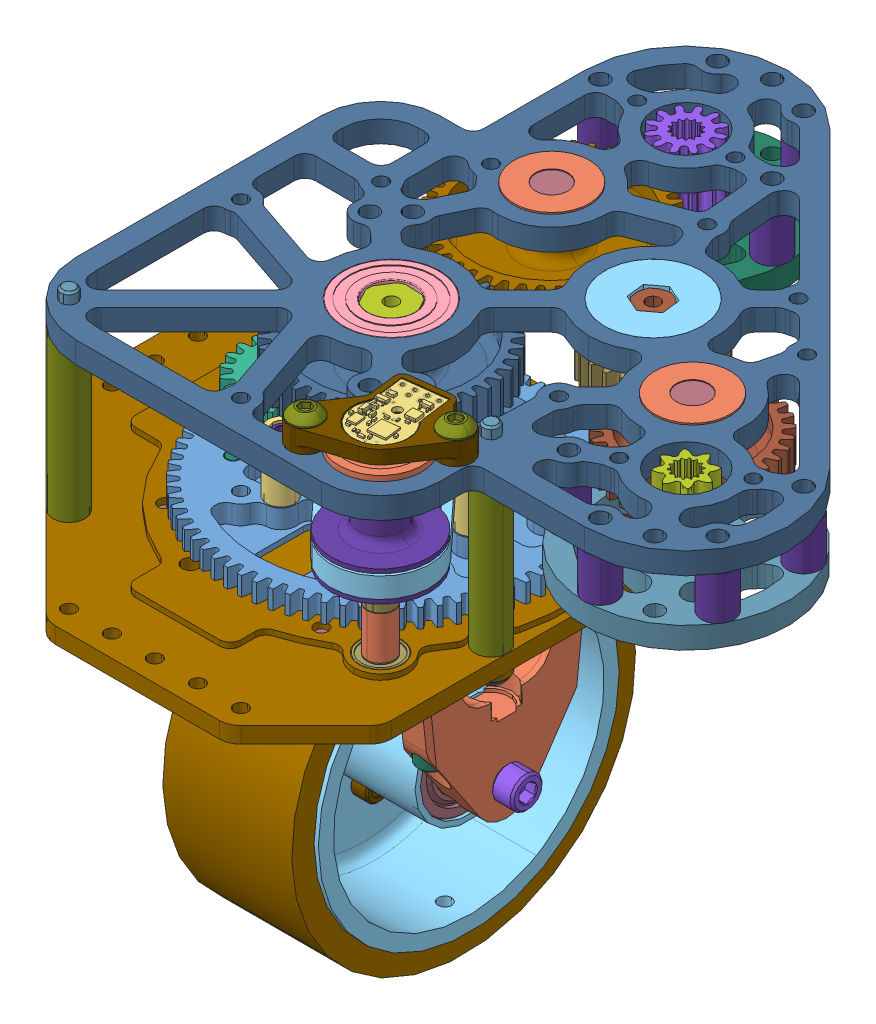
SolidWorks assembly WCP-0361 - Swerve X (Tube Mount, Flipped Gears Below) (WCP-0363).step-1, configuration Default. Lengths in mm.
Overall size (208.72 184.42 201.03).
94 component instances, 59 part files, 0 mates.
Components (placement in the parent):
- WCP-0364 Rev1 - WCP X Wheel Module.step-1-1: WCP-0364 Rev1 - WCP X Wheel Module.step-1 [Default] at (0 -0.825 0) size (95.62 174.54 137.74)
  - WCP-0364-001 Rev1.step-1-1: WCP-0364-001 Rev1.step-1 [Default] at (0 6.35 0) size (93.93 9.53 93.93)
  - WCP-0366 Rev1_Default_As Machined_.step-1-1: WCP-0366 Rev1_Default_As Machined_.step-1 [Default] at (29.2862 -49.2125 0) x (0 0 -1) z (1 0 0) size (51.81 60.46 9.5)
  - WCP-0366 Rev1_Default_As Machined_.step-1-2: WCP-0366 Rev1_Default_As Machined_.step-1 [Default] at (-29.2862 -49.2125 0) x (0 0 1) z (-1 0 0) size (51.81 60.46 9.5)
  - WCP-0364-006 Rev1.step-1-1: WCP-0364-006 Rev1.step-1 [Default] at (0 -49.2125 0) x (1 0 0) z (0 -0.837962 0.545729) size (56.46 12.67 12.67)
  - WCP-0364-005 Rev2.step-1-1: WCP-0364-005 Rev2.step-1 [Default] at (-29.2862 -1.2827 0) x (0 -1 0) z (0 0 1) size (54.08 11 11)
  - WCP-0365 Rev2.step-1-1: WCP-0365 Rev2.step-1 [Default] at (2.3061 -49.2125 0) x (0 -0.866025 -0.5) z (1 0 0) size (88.9 88.9 41.15)
  - WCP-0233 Rev1.step-1-1: WCP-0233 Rev1.step-1 [Default] at (-18.0375 -49.2125 0) x (0 0 -1) z (0 1 0) size (68.52 16.32 68.56)
  - WCP-0364-002 Rev1.step-1-1: WCP-0364-002 Rev1.step-1 [Default] at (0 34.5757 0) x (0 -1 0) z (0.999257 0 0.03854) size (51.69 15 15)
  - WCP-0276 Rev1.step-1-1: WCP-0276 Rev1.step-1 [Default] at (-29.2862 -15.4625 0) x (0 0 1) z (1 0 0) size (25.2 12.86 25.34)
  - WCP-0364-008 Rev1.step-1-1: WCP-0364-008 Rev1.step-1 [Default] at (2.3061 -49.2125 0) x (1 0 0) z (0 -0.879106 0.476626) size (38.1 101.6 101.6)
  - WCP-0357 Rev1.step-1-1: WCP-0357 Rev1.step-1 [Default] at origin size (88.91 6.35 88.9)
  - 217-5829_0375_flanged_thunderhex_bearing.step-1-1: 217-5829_0375_flanged_thunderhex_bearing.step-1 [Default] at (-29.2862 12.7 0) x (0 -1 0) z (0.06043 0 0.998172) size (7.11 24.61 24.61)
  - 217-3489_0_250_radial_bearing.step-1-1: 217-3489_0_250_radial_bearing.step-1 [Default] at (-29.2862 -29.3687 0) x (0 -1 0) z (0.460874 0 0.887465) size (4.76 12.7 12.7)
  - 217-3109_0_500_radial_bearing.step-1-1: 217-3109_0_500_radial_bearing.step-1 [Default] at (-17.8424 -49.2125 0) x (1 0 0) z (0 0.040496 0.99918) size (7.94 28.57 28.57)
  - 217-3109_0_500_radial_bearing.step-1-2: 217-3109_0_500_radial_bearing.step-1 [Default] at (18.0604 -49.2125 0) x (1 0 0) z (0 -0.205758 0.978603) size (7.94 28.57 28.57)
  - 217-2731_0_500_flanged_bearing.step-1-1: 217-2731_0_500_flanged_bearing.step-1 [Default] at (0 4.7625 0) x (0.999376 0 -0.035335) z (0.035335 0 0.999376) size (31.12 7.94 31.12)
  - NFS-0018_SHCS_#10-32_1_750L_Default_As Machined_.step-1-1: NFS-0018_SHCS_#10-32_1_750L_Default_As Machined_.step-1 [Default] at (-29.2862 11.1125 17.4625) x (0.988526 0 -0.151053) z (0 1 0) size (7.92 7.92 49.28)
  - NFS-0018_SHCS_#10-32_1_750L_Default_As Machined_.step-1-2: NFS-0018_SHCS_#10-32_1_750L_Default_As Machined_.step-1 [Default] at (-29.2862 11.1125 -17.4625) x (0.988526 0 -0.151053) z (0 1 0) size (7.92 7.92 49.28)
  - NFS-0018_SHCS_#10-32_1_750L_Default_As Machined_.step-1-3: NFS-0018_SHCS_#10-32_1_750L_Default_As Machined_.step-1 [Default] at (29.2862 11.1125 17.4625) x (0.988526 0 -0.151053) z (0 1 0) size (7.92 7.92 49.28)
  - NFS-0018_SHCS_#10-32_1_750L_Default_As Machined_.step-1-4: NFS-0018_SHCS_#10-32_1_750L_Default_As Machined_.step-1 [Default] at (29.2862 11.1125 -17.4625) x (0.988526 0 -0.151053) z (0 1 0) size (7.92 7.92 49.28)
  - 8-32 BHCS_0.500.step-1-1: 8-32 BHCS_0.500.step-1 [Default] at (-29.2862 23.8633 0) x (0.940105 0 -0.340884) z (0.340884 0 0.940105) size (7.92 14.92 7.92)
  - NFS-0059_SHCS_#4-40_0_875L_91251A113.step-1-1: NFS-0059_SHCS_#4-40_0_875L_91251A113.step-1 [Default] at (23.876 3.5687 0) x (0.431119 0 0.902295) z (0 -1 0) size (4.65 4.65 25.08)
  - NFS-0059_SHCS_#4-40_0_875L_91251A113.step-1-2: NFS-0059_SHCS_#4-40_0_875L_91251A113.step-1 [Default] at (23.876 3.0654 0) x (0.520663 0 0.853762) z (0 -1 0) size (4.65 4.65 25.08)
  - NFS-0059_SHCS_#4-40_0_875L_91251A113.step-1-3: NFS-0059_SHCS_#4-40_0_875L_91251A113.step-1 [Default] at (-11.938 3.5687 -20.6772) x (0.431119 0 0.902295) z (0 -1 0) size (4.65 4.65 25.08)
  - NFS-0059_SHCS_#4-40_0_875L_91251A113.step-1-4: NFS-0059_SHCS_#4-40_0_875L_91251A113.step-1 [Default] at (-11.938 3.0654 -20.6772) x (0.520663 0 0.853762) z (0 -1 0) size (4.65 4.65 25.08)
  - NFS-0059_SHCS_#4-40_0_875L_91251A113.step-1-5: NFS-0059_SHCS_#4-40_0_875L_91251A113.step-1 [Default] at (-11.938 3.0654 20.6772) x (0.520663 0 0.853762) z (0 -1 0) size (4.65 4.65 25.08)
  - 10-32 SHCS - No Thread_WCP-0265 - 0.375.step-1-1: 10-32 SHCS - No Thread_WCP-0265 - 0.375.step-1 [Default] at (-8.2862 -59.5312 17.8726) x (0 -0.796051 -0.60523) z (0 -0.60523 0.796051) size (7.67 14.35 7.67)
  - 10-32 SHCS - No Thread_WCP-0265 - 0.375.step-1-2: 10-32 SHCS - No Thread_WCP-0265 - 0.375.step-1 [Default] at (-8.2862 -38.8937 -17.8726) x (0 -0.796051 -0.60523) z (0 -0.60523 0.796051) size (7.67 14.35 7.67)
  - 10-32 SHCS - No Thread_WCP-0265 - 0.375.step-1-3: 10-32 SHCS - No Thread_WCP-0265 - 0.375.step-1 [Default] at (-8.2862 -38.8937 17.8726) x (0 -0.796051 -0.60523) z (0 -0.60523 0.796051) size (7.67 14.35 7.67)
  - 10-32 SHCS - No Thread_WCP-0265 - 0.375.step-1-4: 10-32 SHCS - No Thread_WCP-0265 - 0.375.step-1 [Default] at (-8.2862 -59.5312 -17.8726) x (0 -0.796051 -0.60523) z (0 -0.60523 0.796051) size (7.67 14.35 7.67)
  - 10-32 SHCS - No Thread_WCP-0265 - 0.375.step-1-5: 10-32 SHCS - No Thread_WCP-0265 - 0.375.step-1 [Default] at (-8.2862 -28.575 0) x (0 -0.796051 -0.60523) z (0 -0.60523 0.796051) size (7.67 14.35 7.67)
  - 10-32 SHCS - No Thread_WCP-0265 - 0.375.step-1-6: 10-32 SHCS - No Thread_WCP-0265 - 0.375.step-1 [Default] at (-8.2862 -69.85 0) x (0 0.591573 -0.806252) z (0 -0.806252 -0.591573) size (7.67 14.35 7.67)
  - NFS-0024_250-20_thin_locknut_90566A029.step-1-1: NFS-0024_250-20_thin_locknut_90566A029.step-1 [Default] at (-34.0362 -49.2125 0) x (0 0.824738 0.565516) z (0 -0.565516 0.824738) size (11.14 5.19 12.86)
  - WCP-0229 Rev1.step-1-1: WCP-0229 Rev1.step-1 [Default] at (-22.6822 -49.2125 0) size (0.89 16.1 14.34)
  - WCP-0229 Rev1.step-1-2: WCP-0229 Rev1.step-1 [Default] at (22.6822 -49.2125 0) size (0.89 16.1 14.34)
  - WCP-0367-002 Rev3.step-1-1: WCP-0367-002 Rev3.step-1 [Default] at (0 28.6559 0) x (0 0 -1) z (1 0 0) size (49.74 26.04 44.2)
  - WCP-0367-006 Rev1.step-1-1: WCP-0367-006 Rev1.step-1 [Default] at (-29.2862 -3.81 0) size (17.27 17.14 17.27)
  - WCP-0367-010 Rev1.step-1-1: WCP-0367-010 Rev1.step-1 [Default] at (-29.2862 22.2758 0) x (0 0 1) z (-1 0 0) size (12.7 4.76 12.7)
  - WCP-0434 Rev1.step-1-1: WCP-0434 Rev1.step-1 [Default] at (-29.2862 19 0) x (-0.327758 0 -0.944762) z (0 -1 0) size (30.3 30.48 12.6)
  - 217-5464_24T_500_hex_steel.step-1-1: 217-5464_24T_500_hex_steel.step-1 [Default] at (0 19 0) x (0.428371 0 0.903603) z (0 -1 0) size (32.87 32.87 12.6)
  - 0250-20_3L_SHCS_91251A554.step-1-1: 0250-20_3L_SHCS_91251A554.step-1 [Default] at (-0.8888 -49.2125 0) x (0 -0.133483 -0.991051) z (1 0 0) size (9.53 9.53 82.55)
- 217-3489_0_250_radial_bearing.step-1-1: 217-3489_0_250_radial_bearing.step-1 [Default] at (36.5633 1.6187 39.7383) x (0 1 0) z (-0.269707 0 0.962942) size (4.76 12.7 12.7)
- WCP-0360-001 Rev1.step-1-1: WCP-0360-001 Rev1.step-1 [Default] at origin size (133.35 8 133.35)
- WCP-0361-001 Rev2.step-1-1: WCP-0361-001 Rev2.step-1 [Default] at (0 53.1812 0) size (174.12 6.35 174.12)
- WCP-0364-003 Rev1.step-1-1: WCP-0364-003 Rev1.step-1 [Default] at (38.669 7.5147 -38.669) x (0.682654 0 0.730742) z (0 1 0) size (20.01 20.32 56.54)
- WCP-0364-004 Rev1.step-1-1: WCP-0364-004 Rev1.step-1 [Default] at (36.5633 23.984 39.7383) x (0 1 0) z (-0.373833 0 -0.927496) size (58.72 11 11)
- WCP-0361-004 Rev1_Default_As Machined_.step-1-1: WCP-0361-004 Rev1_Default_As Machined_.step-1 [Default] at (69.0125 43.1356 -19.9819) x (0 -1 0) z (-0.01804 0 -0.999837) size (25.16 11 11)
- WCP-0361-004 Rev1_Default_As Machined_.step-1-2: WCP-0361-004 Rev1_Default_As Machined_.step-1 [Default] at (-5.7166 43.1356 -53.1094) x (0 -1 0) z (0.932067 0 0.362285) size (25.16 11 11)
- WCP-0361-005 Rev1.step-1-1: WCP-0361-005 Rev1.step-1 [Default] at (86.9695 34.1313 -0.16) x (0.741112 0 -0.671382) z (0.671382 0 0.741112) size (60 6.35 71.67)
- WCP-0361-002 Rev1.step-1-1: WCP-0361-002 Rev1.step-1 [Default] at (0.16 34.1313 -86.9695) x (-0.985271 0 -0.170999) z (0.170999 0 -0.985271) size (60 6.35 79.29)
- WCP-0387 Rev1.step-1-1: WCP-0387 Rev1.step-1 [Default] at (49.2125 26.1937 19.7361) x (0 -1 0) z (0.97467 0 0.223647) size (47.62 9.5 9.5)
- WCP-0387 Rev1.step-1-2: WCP-0387 Rev1.step-1 [Default] at (-47.625 26.1937 47.625) x (0 -1 0) z (-0.427741 0 0.903901) size (47.62 9.5 9.5)
- WCP-0202 Rev1.step-1-1: WCP-0202 Rev1.step-1 [Default] at (-12.54 43.6562 -108.9665) x (0 -1 0) z (0.721842 0 0.692058) size (12.7 9.5 9.5)
- WCP-0202 Rev1.step-1-2: WCP-0202 Rev1.step-1 [Default] at (108.9665 43.6562 -12.86) x (0 -1 0) z (0.721842 0 0.692058) size (12.7 9.5 9.5)
- WCP-0202 Rev1.step-1-3: WCP-0202 Rev1.step-1 [Default] at (64.9724 43.6562 12.54) x (0 -1 0) z (0.721842 0 0.692058) size (12.7 9.5 9.5)
- WCP-0202 Rev1.step-1-4: WCP-0202 Rev1.step-1 [Default] at (25.56 43.6562 -86.9695) x (0 -1 0) z (0.721842 0 0.692058) size (12.7 9.5 9.5)
- WCP-0202 Rev1.step-1-5: WCP-0202 Rev1.step-1 [Default] at (86.9695 43.6562 25.24) x (0 -1 0) z (0.721842 0 0.692058) size (12.7 9.5 9.5)
- WCP-0202 Rev1.step-1-6: WCP-0202 Rev1.step-1 [Default] at (-25.24 43.6562 -86.9695) x (0 -1 0) z (0.721842 0 0.692058) size (12.7 9.5 9.5)
- WCP-0202 Rev1.step-1-7: WCP-0202 Rev1.step-1 [Default] at (12.86 43.6562 -108.9665) x (0 -1 0) z (0.721842 0 0.692058) size (12.7 9.5 9.5)
- WCP-0202 Rev1.step-1-8: WCP-0202 Rev1.step-1 [Default] at (108.9665 43.6562 12.54) x (0 -1 0) z (0.721842 0 0.692058) size (12.7 9.5 9.5)
- WCP-0226 Rev1.step-1-1: WCP-0226 Rev1.step-1 [Default] at (-19.7361 16.6687 -49.2125) x (0 1 0) z (0.900957 0 0.433909) size (28.57 9.5 9.5)
- WCP-0307 Rev1.step-1-1: WCP-0307 Rev1.step-1 [Default] at (-19.7361 -5.5913 -49.2125) x (0 -1 0) z (-0.403935 0 0.914788) size (3.18 9.5 9.5)
- 217-2733_0_375_flanged_bearing.step-1-1: 217-2733_0_375_flanged_bearing.step-1 [Default] at (69.0125 49.6887 -19.9819) x (0 1 0) z (0.053261 0 -0.998581) size (7.11 24.61 24.61)
- 217-2733_0_375_flanged_bearing.step-1-2: 217-2733_0_375_flanged_bearing.step-1 [Default] at (36.5633 57.9438 39.7383) x (0 -1 0) z (0.710471 0 -0.703726) size (7.11 24.61 24.61)
- 217-2733_0_375_flanged_bearing.step-1-3: 217-2733_0_375_flanged_bearing.step-1 [Default] at (-5.7166 49.6887 -53.1094) x (0 1 0) z (0.053261 0 -0.998581) size (7.11 24.61 24.61)
- WCP-0041_0_250_radial_bearing.step-1-1: WCP-0041_0_250_radial_bearing.step-1 [Default] at (38.669 1.5108 -38.669) x (-0.316483 0 0.948598) z (0 -1 0) size (15.88 15.88 4.98)
- 217-4006_0_500_flanged_thunderhex_bearing.step-1-1: 217-4006_0_500_flanged_thunderhex_bearing.step-1 [Default] at (0 52.3875 0) x (-0.903668 0 0.428233) z (0 -1 0) size (31.12 31.12 7.94)
- 217-2735_0_375_flanged_hex_bearing.step-1-1: 217-2735_0_375_flanged_hex_bearing.step-1 [Default] at (38.669 56.3562 -38.669) x (-0.91814 0 -0.396256) z (-0.396256 0 0.91814) size (31.12 7.94 31.12)
- WCP-0042_0_250_flanged_bearing.step-1-1: WCP-0042_0_250_flanged_bearing.step-1 [Default] at (69.0125 33.8899 -19.9819) x (0.753109 0 -0.657896) z (0 1 0) size (18.24 18.24 4.98)
- WCP-0042_0_250_flanged_bearing.step-1-2: WCP-0042_0_250_flanged_bearing.step-1 [Default] at (-5.7166 33.8899 -53.1094) x (0.890667 0 -0.454657) z (0 1 0) size (18.24 18.24 4.98)
- 217-6915_Falcon_8T.step-1-1: 217-6915_Falcon_8T.step-1 [Default] at (86.9695 46.7088 -0.16) x (0.340812 0 -0.940132) z (0 -1 0) size (13.62 13.62 19.06)
- 217-6919_Falcon_12T.step-1-1: 217-6919_Falcon_12T.step-1 [Default] at (0.16 46.7088 -86.9695) x (-0.557793 0 0.82998) z (0 -1 0) size (17.78 17.78 19.05)
- WCP-0541 Rev1.step-1-1: WCP-0541 Rev1.step-1 [Default] at (-5.7166 43.1482 -53.1094) x (0.992001 0 0.126228) z (0 1 0) size (55.8 55.88 12.65)
- WCP-0178 Rev1.step-1-1: WCP-0178 Rev1.step-1 [Default] at (0 42.0941 0) x (0.993242 0 -0.116064) z (0 1 0) size (55.8 55.88 12.65)
- WCP-0540 Rev1.step-1-1: WCP-0540 Rev1.step-1 [Default] at (69.0125 43.1236 -19.9819) x (0.992415 0 -0.122933) z (0 1 0) size (43.07 43.07 12.6)
- WCP-0538 Rev1.step-1-1: WCP-0538 Rev1.step-1 [Default] at (38.669 41.9158 -38.669) x (0.27049 0 -0.962723) z (0 1 0) size (32.86 32.86 12.65)
- 10-32 BHCS - No Thread_WCP-0251 - 0.250.step-1-1: 10-32 BHCS - No Thread_WCP-0251 - 0.250.step-1 [Default] at (-33.4155 -4 33.4155) x (0.140263 0 -0.990114) z (-0.990114 0 -0.140263) size (9.17 8.92 9.17)
- 10-32 BHCS - No Thread_WCP-0251 - 0.250.step-1-2: 10-32 BHCS - No Thread_WCP-0251 - 0.250.step-1 [Default] at (7.3926 -4 -46.6749) x (0.4685 0 0.883464) z (0.883464 0 -0.4685) size (9.17 8.92 9.17)
- 10-32 BHCS - No Thread_WCP-0251 - 0.250.step-1-3: 10-32 BHCS - No Thread_WCP-0251 - 0.250.step-1 [Default] at (46.6749 -4 -7.3926) x (-0.69545 0 0.718575) z (0.718575 0 0.69545) size (9.17 8.92 9.17)
- 10-32 BHCS - No Thread_WCP-0251 - 0.250.step-1-4: 10-32 BHCS - No Thread_WCP-0251 - 0.250.step-1 [Default] at (-42.106 -4 -21.4541) x (0.984998 0 -0.172564) z (-0.172564 0 -0.984998) size (9.17 8.92 9.17)
- 10-32 BHCS - No Thread_WCP-0251 - 0.250.step-1-5: 10-32 BHCS - No Thread_WCP-0251 - 0.250.step-1 [Default] at (21.4541 -4 42.106) x (-0.898311 0 -0.43936) z (-0.43936 0 0.898311) size (9.17 8.92 9.17)
- 10-32 BHCS - No Thread_WCP-0261 - 2.500.step-1-1: 10-32 BHCS - No Thread_WCP-0261 - 2.500.step-1 [Default] at (49.2125 -4 19.7361) x (0.670106 0 -0.742266) z (-0.742266 0 -0.670106) size (9.17 66.07 9.17)
- 10-32 BHCS - No Thread_WCP-0261 - 2.500.step-1-2: 10-32 BHCS - No Thread_WCP-0261 - 2.500.step-1 [Default] at (-47.625 -4 47.625) x (0.958479 0 -0.285162) z (-0.285162 0 -0.958479) size (9.17 66.07 9.17)
- 10-32 BHCS - No Thread_WCP-0258 - 1.750.step-1-1: 10-32 BHCS - No Thread_WCP-0258 - 1.750.step-1 [Default] at (-19.7361 -7.175 -49.2125) x (0.978856 0 -0.204553) z (-0.204553 0 -0.978856) size (9.17 47.02 9.17)
- 10-32 BHCS - No Thread_WCP-0253 - 0.500.step-1-1: 10-32 BHCS - No Thread_WCP-0253 - 0.500.step-1 [Default] at (23.914 62.9348 49.3306) x (-0.153016 0 -0.988224) z (0.988224 0 -0.153016) size (9.17 15.27 9.17)
- 10-32 BHCS - No Thread_WCP-0253 - 0.500.step-1-2: 10-32 BHCS - No Thread_WCP-0253 - 0.500.step-1 [Default] at (49.2125 62.9348 30.146) x (0.162273 0 -0.986746) z (0.986746 0 0.162273) size (9.17 15.27 9.17)
- WCP-0367-003 Rev2.step-1-1: WCP-0367-003 Rev2.step-1 [Default] at (36.5633 25.8309 39.7383) x (-0.999998 0 0.001857) z (0 -1 0) size (29.05 29.05 26.83)
- WCP-0367-012 Rev1_30 Left.step-1-1: WCP-0367-012 Rev1_30 Left.step-1 [Default] at (36.5633 60.9155 39.7383) x (-0.992171 0 0.124885) z (-0.124885 0 -0.992171) size (37.02 6.58 29.76)
- WCP-0367-001 Rev1.step-1-1: WCP-0367-001 Rev1.step-1 [Default] at (0 35.3446 0) x (0.987744 0 0.156082) z (-0.156082 0 0.987744) size (19.05 0.51 19.05)
- WCP-0367-004 Rev1.step-1-1: WCP-0367-004 Rev1.step-1 [Default] at (36.5633 10.35 39.7383) size (8 12.7 8)
- CANcoder.step-1-1: CANcoder.step-1 [Default] at (36.5485 59.1546 39.7225) x (-0.992171 0 0.124885) z (0 1 0) size (15.94 23.28 4.54)
- WCP-0156 Rev1.step-1-1: WCP-0156 Rev1.step-1 [Default] at (36.5633 51.5938 39.7383) size (6.35 12.7 6.35)
- Encoder Belt.step-1-1: Encoder Belt.step-1 [Default] at (18.2816 30.8309 19.8691) x (0.677097 0 0.735894) z (-0.735894 0 0.677097) size (83.28 6 29.28)
